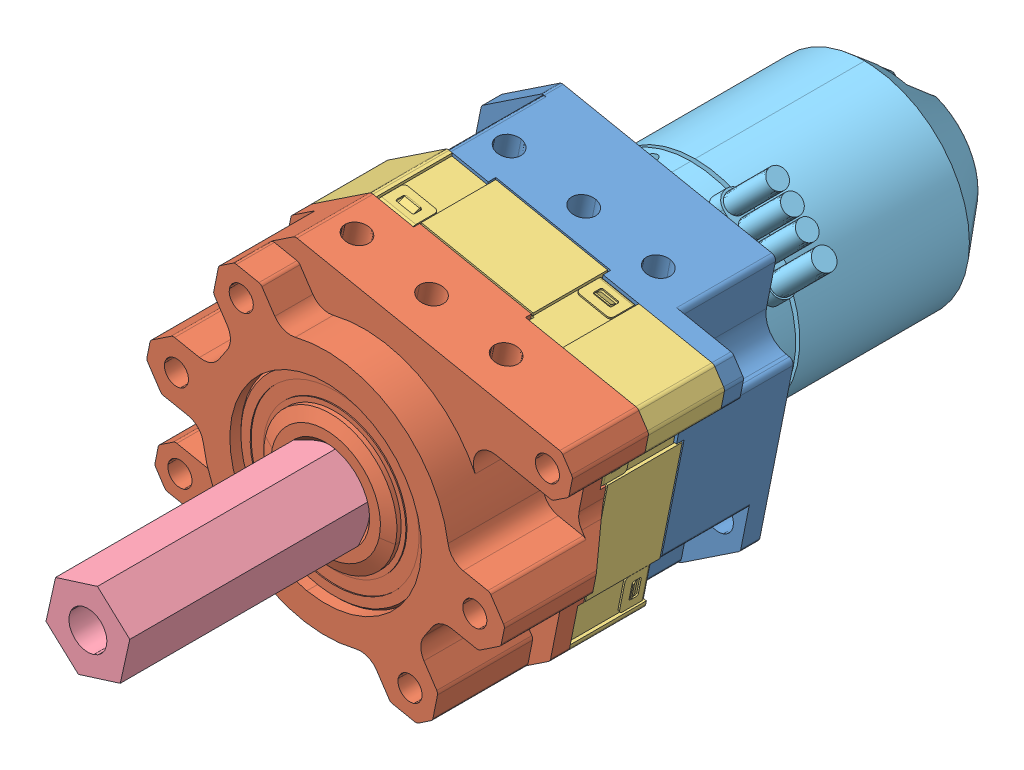
SolidWorks assembly Neo_550_with_1_Stage_Gearbox, configuration Default. Lengths in mm.
Overall size (70.69 61.96 138.17).
5 component instances, 5 part files, 20 mates.
Components (placement in the parent):
- REV-21-2106.step-1: REV-21-2106.step [Default] at (-1.1023 -0.9864 127.25) x (0.980561 -0.196216 0) z (0 0 1) size (61.91 50.8 19.05)
- REV-21-2104.step-1: REV-21-2104.step [Default] at (-1.1023 -0.9864 159) x (0 0 1) z (-0.980561 0.196216 0) size (23.2 50.8 61.92)
- REV-21-2103.step-2: REV-21-2103.step [Default] at (-1.1023 -0.9864 143.125) x (0.980561 -0.196216 0) z (0 0 1) size (61.91 50.8 16.85)
- motor_drive_shaft-1: motor_drive_shaft [Default] at (-1.1023 -0.9864 157.4125) x (0.217469 0.976067 0) z (0 0 1) size (14.66 12.7 50.8)
- REV-21-1651.STEP-1: REV-21-1651.STEP [Default] at (-1.1023 -0.9864 126.05) x (0 0 -1) z (1 0 0) size (56.01 42.91 43.01)
Mates (geometry in assembly coordinates):
- Concentric2: concentric aligned: circle of REV-21-2103.step-1; circle of REV-21-2103.step-2
- Concentric3: concentric anti-aligned: circle of REV-21-2104.step-1; circle of REV-21-2103.step-2
- Concentric4: concentric anti-aligned: circle of REV-21-1650-V1.1.step-1; circle of REV-21-2106.step-1
- Concentric5: concentric anti-aligned: circle of REV-21-1650-V1.1.step-1; circle of REV-21-2106.step-1
- Parallel2: parallel aligned: plane of REV-21-2103.step-1 through (18.82 -30.8765 136.775) normal (0.980561 -0.196216 0); plane of REV-21-2103.step-2 through (18.82 -30.8765 149.475) normal (0.980561 -0.196216 0)
- Parallel3: parallel aligned: plane of REV-21-2104.step-1 through (18.82 -30.8765 149.475) normal (-0.196216 -0.980561 0); plane of REV-21-2103.step-2 through (18.82 -30.8765 149.475) normal (-0.196216 -0.980561 0)
- Coincident6: coincident anti-aligned: plane of REV-21-1650-V1.1.step-1 through (-1.1023 -0.9864 105.025) normal (0 0 1); plane of REV-21-2106.step-1 through (-1.1023 -0.9864 117.725) normal (0 0 -1)
- Coincident8: coincident anti-aligned: plane of REV-21-2103.step-1 through (-1.1023 -0.9864 136.775) normal (0 0 1); plane of REV-21-2103.step-2 through (-1.1023 -0.9864 136.775) normal (0 0 -1)
- Coincident9: coincident anti-aligned: plane of REV-21-2104.step-1 through (-1.1023 -0.9864 149.475) normal (0 0 -1); plane of REV-21-2103.step-2 through (-1.1023 -0.9864 149.475) normal (0 0 1)
- Concentric6: concentric aligned: circle of REV-21-2104.step-1; circle of motor_drive_shaft-1
- Coincident10: coincident anti-aligned: plane of REV-21-2104.step-1 through (-1.1023 -0.9864 157.4125) normal (0 0 1); plane of motor_drive_shaft-1 through (-1.1023 -0.9864 157.4125) normal (0 0 -1)
- Parallel4: parallel aligned: plane of REV-21-2104.step-1 through (-2.6985 -8.1504 157.4125) normal (-0.2997 0.954033 0); plane of motor_drive_shaft-1 through (0.4922 6.1705 208.2125) normal (-0.2997 0.954033 0)
- Coincident11: coincident anti-aligned: plane of REV-21-2103.step-2 through (-1.1023 -0.9864 136.775) normal (0 0 -1); plane of REV-21-2103.step-3 through (-1.1023 -0.9864 136.775) normal (0 0 1)
- Concentric7: concentric anti-aligned: circle of REV-21-2106.step-1; circle of REV-21-2103.step-3
- Parallel5: parallel aligned: plane of REV-21-2103.step-2 through (28.7878 18.936 149.475) normal (0.196216 0.980561 0); plane of REV-21-2103.step-3 through (28.7878 18.936 136.775) normal (0.196216 0.980561 0)
- Concentric8: concentric aligned: circle of REV-21-2106.step-1; circle of REV-21-2103.step-2
- Coincident12: coincident anti-aligned: plane of REV-21-2106.step-1 through (-1.1023 -0.9864 136.775) normal (0 0 1); plane of REV-21-2103.step-2 through (-1.1023 -0.9864 136.775) normal (0 0 -1)
- Parallel6: parallel aligned: plane of REV-21-2106.step-1 through (3.8815 23.9199 136.775) normal (0.196216 0.980561 0); plane of REV-21-2103.step-2 through (28.7878 18.936 149.475) normal (0.196216 0.980561 0)
- Concentric9: concentric aligned: circle of REV-21-2106.step-1; circle of REV-21-1651.STEP-1
- Distance1: distance = 3.175 mm anti-aligned: plane of REV-21-2106.step-1 through (-1.1023 -0.9864 117.725) normal (0 0 -1); plane of REV-21-1651.step-1 through (-1.1023 5.5136 114.55) normal (0 0 1)
